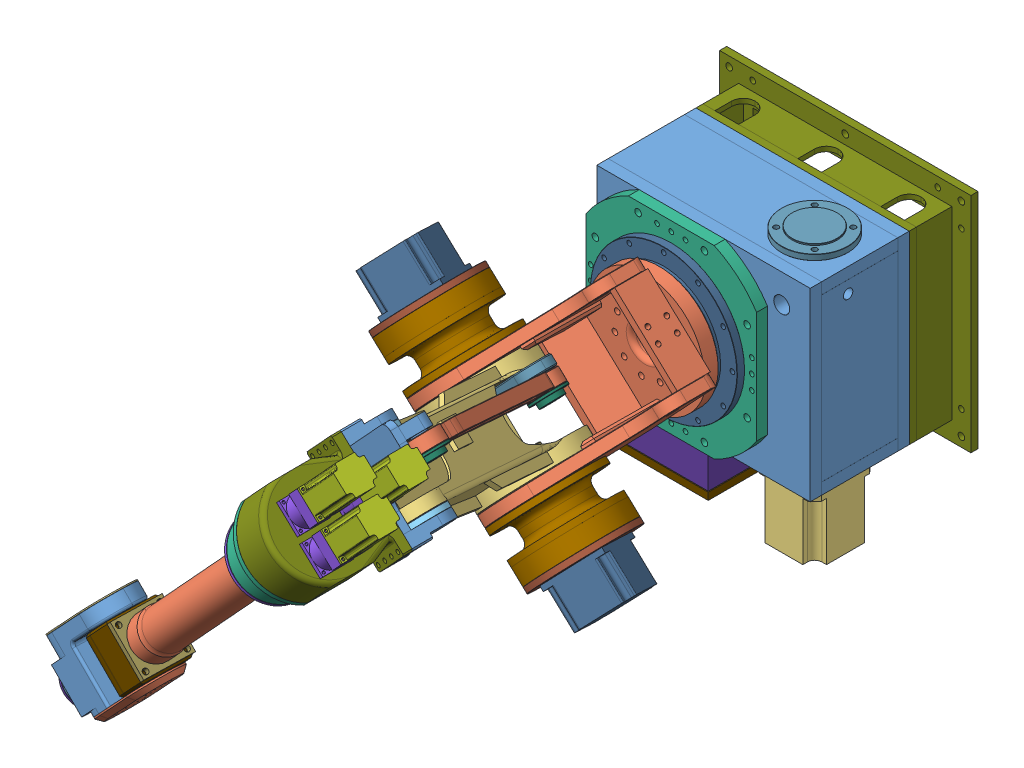
SolidWorks assembly CHX-3装配图, configuration 默认. Lengths in mm. (continued)
Mates (geometry in assembly coordinates): (continued)
- 同心322: concentric aligned: cylinder of CHX-3腕部中心轴2-1 through (-292.5541 -282.9044 1255.4054) axis (0.677165 0.724539 0.128414) radius 7.5; cylinder of CHX-3手腕61902轴承-2 through (-274.4738 -263.5592 1258.8341) axis (0.677165 0.724539 0.128414) radius 14
- 重合247: coincident anti-aligned: plane of CHX-3手腕61902轴承-1 through (-269.7336 -258.4875 1259.733) normal (-0.677165 -0.724539 -0.128414); plane of CHX-3手腕61902轴承-2
- 同心323: concentric anti-aligned: cylinder of CHX-3腕部中心轴1-2 through (-228.9006 -214.7978 1267.4764) axis (-0.677165 -0.724539 -0.128414) radius 34; cylinder of CHK-3前爪固定座-2 through (-246.5068 -233.6358 1264.1376) axis (0.677165 0.724539 0.128414) radius 34
- 同心324: concentric aligned: cylinder of CHK-3前爪固定座-2 through (-241.2095 -229.1944 1226.7182) axis (-0.677165 -0.724539 -0.128414) radius 3; cylinder of CHX-3腕部中心轴1-2 through (-232.4063 -219.7754 1228.3876) axis (-0.677165 -0.724539 -0.128414) radius 2
- 重合248: coincident anti-aligned: plane of CHX-3腕部中心轴1-2 through (-246.5068 -233.6358 1264.1376) normal (-0.677165 -0.724539 -0.128414); plane of CHK-3前爪固定座-2 through (-215.2712 -271.8091 1314.8045) normal (0.677165 0.724539 0.128414)
- 同心328: concentric anti-aligned: cylinder of CHX-3腕部中心轴2-1 through (-292.5541 -282.9044 1255.4054) axis (0.677165 0.724539 0.128414) radius 7.5; cylinder of CHX-3手腕小齿-1 through (-274.4738 -263.5592 1258.8341) axis (-0.677165 -0.724539 -0.128414) radius 16
- 重合254: coincident anti-aligned: plane of CHX-3手腕61902轴承-2; plane of CHX-3手腕小齿-1 through (-274.4738 -263.5592 1258.8341) normal (0.677165 0.724539 0.128414)
- 重合261: coincident anti-aligned: plane of CHK-3前爪固定座-2 through (-223.3972 -280.5036 1313.2635) normal (-0.677165 -0.724539 -0.128414); plane of CHK-3前爪法兰-1 through (-306.234 -203.5239 1315.7509) normal (0.677165 0.724539 0.128414)
- 同心334: concentric aligned: cylinder of CHK-3前爪固定座-2 through (-254.6328 -242.3303 1262.5966) axis (0.677165 0.724539 0.128414) radius 30.5; cylinder of CHK-3前爪法兰-1 through (-293.2313 -283.629 1255.277) axis (0.677165 0.724539 0.128414) radius 42.5
- 重合264: coincident: plane of CHK-3前爪固定座-2 through (-223.3972 -280.5036 1313.2635) normal (-0.103765 -0.078746 0.99148); line of CHK-3前爪法兰-1 through (-296.245 -212.0315 1311.0777) axis (0.728478 -0.68472 0.021858)
- 同心336: concentric aligned: cylinder of CHK-3前爪法兰-1 through (-263.3637 -311.7025 1256.1732) axis (-0.728478 0.68472 -0.021858) radius 42.5; cylinder of CHX-3手腕前端旋转法兰-1 through (-341.3108 -238.4374 1253.8344) axis (-0.728478 0.68472 -0.021858) radius 47.75
- 距离41: distance = 1 mm anti-aligned: plane of CHK-3前爪法兰-1 through (-376.2015 -295.1143 1190.2088) normal (-0.728478 0.68472 -0.021858); plane of CHX-3手腕前端旋转法兰-1 through (-289.071 -201.0754 1186.4442) normal (0.728478 -0.68472 0.021858)
- 同心338: concentric anti-aligned: cylinder of CHX-3手腕前端旋转法兰-1 through (-282.652 -416.9987 1254.0099) axis (-0.728478 0.68472 -0.021858) radius 27.5; cylinder of CHK-3前爪法兰侧盖-1 through (-314.705 -386.871 1253.0482) axis (0.728478 -0.68472 0.021858) radius 55
- 同心340: concentric aligned: cylinder of CHX-3手腕前端旋转法兰-1 through (-282.652 -416.9987 1254.0099) axis (-0.728478 0.68472 -0.021858) radius 27.5; cylinder of CHK-3前爪法兰侧钣金盖-1 through (-417.4204 -290.3254 1249.9662) axis (-0.728478 0.68472 -0.021858) radius 55
- 重合267: coincident anti-aligned: plane of CHX-3手腕前端旋转法兰-1 through (-320.5842 -185.3703 1310.4408) normal (-0.728478 0.68472 -0.021858); plane of CHK-3前爪法兰侧钣金盖-1 through (-417.4204 -290.3254 1249.9662) normal (0.728478 -0.68472 0.021858)
- 同心341: concentric aligned: cylinder of CHX-3手腕前端旋转法兰-1 through (-355.8804 -224.743 1253.3972) axis (-0.728478 0.68472 -0.021858) radius 55; cylinder of CHK-3前爪法兰侧钣金盖-1 through (-355.8804 -224.743 1253.3972) axis (-0.728478 0.68472 -0.021858) radius 55
- 同心342: concentric anti-aligned: cylinder of CHX-3手腕前端旋转法兰-1 through (-323.0988 -255.5554 1254.3808) axis (-0.728478 0.68472 -0.021858) radius 17.5; cylinder of CHX-3小手腕旋转齿轮-2 through (-371.1784 -210.3639 1252.9382) axis (0.728478 -0.68472 0.021858) radius 8.5
- 同心344: concentric aligned: cylinder of CHX-3手腕前端旋转法兰-1 through (-323.0988 -255.5554 1254.3808) axis (-0.728478 0.68472 -0.021858) radius 17.5; cylinder of CHX-3手腕大齿-2-1 through (-324.5558 -254.186 1254.3371) axis (-0.728478 0.68472 -0.021858) radius 27.5
- 重合271: coincident aligned: plane of CHK-3前爪法兰-1 through (-324.5558 -254.186 1254.3371) normal (-0.728478 0.68472 -0.021858); plane of CHX-3手腕大齿-2-1 through (-324.5558 -254.186 1254.3371) normal (-0.728478 0.68472 -0.021858)
- 同心345: concentric aligned: cylinder of CHX-3手腕前端旋转法兰-1 through (-337.9277 -242.8472 1277.4428) axis (-0.728478 0.68472 -0.021858) radius 5; cylinder of CHX-3手腕大齿-2-1 through (-323.3581 -256.5416 1277.88) axis (-0.728478 0.68472 -0.021858) radius 2
- 距离44: distance = 1 mm anti-aligned: plane of CHX-3手腕前端旋转法兰-1 through (-341.3108 -238.4374 1253.8344) normal (-0.728478 0.68472 -0.021858); plane of CHX-3小手腕旋转齿轮-2 through (-342.0393 -237.7527 1253.8125) normal (0.728478 -0.68472 0.021858)
- 同心347: concentric aligned: cylinder of CHX-3手腕大齿-2-1 through (-315.8141 -262.4026 1254.5994) axis (0.728478 -0.68472 0.021858) radius 17; cylinder of CHX-3手腕轴1-1 through (-352.9664 -227.4819 1253.4846) axis (0.728478 -0.68472 0.021858) radius 8.5
- 同心348: concentric aligned: cylinder of CHK-3前爪法兰-1 through (-261.9067 -313.072 1256.2169) axis (0.728478 -0.68472 0.021858) radius 45; cylinder of CHK-3前爪法兰侧盖-1 through (-253.165 -321.2886 1256.4792) axis (0.728478 -0.68472 0.021858) radius 55
- 同心349: concentric anti-aligned: cylinder of CHK-3前爪法兰-1 through (-261.9067 -313.072 1256.2169) axis (0.728478 -0.68472 0.021858) radius 45; cylinder of CHX-3手腕前爪连接轴-1 through (-253.8934 -320.6039 1256.4573) axis (-0.728478 0.68472 -0.021858) radius 27.5
- 重合277: coincident anti-aligned: plane of CHK-3前爪法兰-1 through (-261.9067 -313.072 1256.2169) normal (0.728478 -0.68472 0.021858); plane of CHX-3手腕前爪连接轴-1 through (-261.9067 -313.072 1256.2169) normal (-0.728478 0.68472 -0.021858)
- 重合278: coincident anti-aligned: plane of CHK-3前爪法兰侧盖-1 through (-248.0656 -326.0817 1256.6322) normal (-0.728478 0.68472 -0.021858); plane of CHX-3手腕前爪连接轴-1 through (-248.0656 -326.0817 1256.6322) normal (0.728478 -0.68472 0.021858)
- 同心350: concentric aligned: cylinder of CHK-3前爪法兰侧盖-1 through (-250.8925 -292.5681 1256.9435) axis (0.728478 -0.68472 0.021858) radius 3; cylinder of CHX-3手腕前爪连接轴-1 through (-243.6078 -299.4153 1257.1621) axis (0.728478 -0.68472 0.021858) radius 2.5
- 重合279: coincident aligned: plane of CHX-3手腕大齿-2-1 through (-315.8141 -262.4026 1254.5994) normal (-0.728478 0.68472 -0.021858); plane of CHX-3手腕轴1-1 through (-315.8141 -262.4026 1254.5994) normal (-0.728478 0.68472 -0.021858)
- 齿轮配合14: gear = 0.001 : 0.001: cone of CHX-3手腕大齿2-1 through (-267.0771 -255.6451 1260.2367) axis (-0.677165 -0.724539 -0.128414); cone of CHX-3手腕大齿-2-1 through (-321.2944 -257.2515 1254.435) axis (0.728478 -0.68472 0.021858)
- 重合281: coincident aligned: plane of CHX-3小手腕旋转齿轮-2 through (-363.376 -216.9427 1244.316) normal (0.638355 0.690038 0.341101); plane of CHX-3手腕轴1-1 through (-341.3661 -237.3375 1244.3834) normal (0.638355 0.690038 0.341101)
- 同心352: concentric anti-aligned: cylinder of CHX-3手腕前端旋转法兰-1 through (-358.1902 -352.8548 1251.6553) axis (-0.683779 -0.728693 -0.038123) radius 30; cylinder of CHX-3手腕前端锥齿2-1 through (-380.0711 -376.173 1250.4354) axis (0.683779 0.728693 0.038123) radius 19.9123
- 距离45: distance = 18 mm aligned: plane of CHX-3手腕前端旋转法兰-1 through (-427.4724 -359.1824 1303.7125) normal (-0.683779 -0.728693 -0.038123); plane of CHX-3手腕前端锥齿2-1 through (-380.0711 -376.173 1250.4354) normal (-0.683779 -0.728693 -0.038123)
- 同心354: concentric aligned: cylinder of CHX-3手腕前端旋转法兰-1 through (-282.652 -416.9987 1254.0099) axis (-0.728478 0.68472 -0.021858) radius 27.5; cylinder of CHX-3小手腕旋转齿轮-2-1 through (-385.3674 -320.4531 1250.9279) axis (-0.728478 0.68472 -0.021858) radius 17.5
- 重合284: coincident aligned: plane of CHX-3小手腕旋转齿轮-2 through (-352.9664 -227.4819 1253.4846) normal (-0.728478 0.68472 -0.021858); plane of CHX-3小手腕旋转齿轮-2-1 through (-414.5065 -293.0643 1250.0536) normal (-0.728478 0.68472 -0.021858)
- 齿轮配合16: gear = 0.094 : 0.094: cylinder of CHX-3小手腕旋转齿轮-2 through (-342.0393 -237.7527 1253.8125) axis (-0.728478 0.68472 -0.021858) radius 47; cylinder of CHX-3小手腕旋转齿轮-2-1 through (-414.5065 -293.0643 1250.0536) axis (0.728478 -0.68472 0.021858) radius 47
- 同心357: concentric aligned: cylinder of CHX-3手腕前端旋转法兰-1 through (-282.652 -416.9987 1254.0099) axis (-0.728478 0.68472 -0.021858) radius 27.5; cylinder of CHX-3小手腕锥齿轮旋转中心轴-1 through (-381.725 -323.8767 1251.0372) axis (-0.728478 0.68472 -0.021858) radius 17.5
- 重合286: coincident aligned: plane of CHX-3小手腕旋转齿轮-2-1 through (-414.5065 -293.0643 1250.0536) normal (-0.728478 0.68472 -0.021858); plane of CHX-3小手腕锥齿轮旋转中心轴-1 through (-414.5065 -293.0643 1250.0536) normal (-0.728478 0.68472 -0.021858)
- 同心358: concentric anti-aligned: cylinder of CHX-3手腕前端旋转法兰-1 through (-331.46 -371.1224 1252.5454) axis (0.728478 -0.68472 0.021858) radius 23.5; cylinder of CHX-3手腕6204轴承-1 through (-318.3474 -383.4474 1252.9389) axis (-0.728478 0.68472 -0.021858) radius 23.5
- 重合287: coincident anti-aligned: plane of CHX-3手腕前端旋转法兰-1 through (-328.5461 -373.8613 1252.6329) normal (0.728478 -0.68472 0.021858); plane of CHX-3手腕6204轴承-1 through (-328.5461 -373.8613 1252.6329) normal (-0.728478 0.68472 -0.021858)
- 同心359: concentric anti-aligned: cylinder of CHX-3手腕前端旋转法兰-1 through (-395.5661 -310.867 1250.6219) axis (-0.728478 0.68472 -0.021858) radius 31; cylinder of CHX-3手腕6007轴承-1 through (-402.1224 -304.7045 1250.4252) axis (0.728478 -0.68472 0.021858) radius 17.5
- 重合288: coincident anti-aligned: plane of CHX-3手腕前端旋转法兰-1 through (-395.5661 -310.867 1250.6219) normal (-0.728478 0.68472 -0.021858); plane of CHX-3手腕6007轴承-1 through (-395.5661 -310.867 1250.6219) normal (0.728478 -0.68472 0.021858)
- 同心360: concentric anti-aligned: cylinder of CHK-3前爪法兰-1 through (-261.9067 -313.072 1256.2169) axis (0.728478 -0.68472 0.021858) radius 45; cylinder of CHX-3手腕16011轴承-1 through (-253.8934 -320.6039 1256.4573) axis (-0.728478 0.68472 -0.021858) radius 27.5
- 重合289: coincident anti-aligned: plane of CHK-3前爪法兰-1 through (-261.9067 -313.072 1256.2169) normal (0.728478 -0.68472 0.021858); plane of CHX-3手腕16011轴承-1 through (-261.9067 -313.072 1256.2169) normal (-0.728478 0.68472 -0.021858)
- 同心361: concentric aligned: cylinder of CHK-3前爪法兰-1 through (-324.5558 -254.186 1254.3371) axis (-0.728478 0.68472 -0.021858) radius 45; cylinder of CHX-3手腕16011轴承-2 through (-324.5558 -254.186 1254.3371) axis (-0.728478 0.68472 -0.021858) radius 27.5
- 重合290: coincident anti-aligned: plane of CHK-3前爪法兰-1 through (-324.5558 -254.186 1254.3371) normal (-0.728478 0.68472 -0.021858); plane of CHX-3手腕16011轴承-2 through (-324.5558 -254.186 1254.3371) normal (0.728478 -0.68472 0.021858)
- 同心362: concentric aligned: cylinder of CHX-3手腕前端旋转法兰-1 through (-375.2847 -371.0721 1250.7023) axis (-0.683779 -0.728693 -0.038123) radius 34; cylinder of CHX-3小手腕前端法兰-1 through (-376.6523 -372.5295 1250.626) axis (-0.683779 -0.728693 -0.038123) radius 34
- 重合292: coincident anti-aligned: plane of CHX-3手腕前端旋转法兰-1 through (-427.4724 -359.1824 1303.7125) normal (-0.683779 -0.728693 -0.038123); plane of CHX-3小手腕前端法兰-1 through (-392.3792 -389.2895 1249.7492) normal (0.683779 0.728693 0.038123)
- 同心364: concentric anti-aligned: cylinder of CHX-3手腕前端旋转法兰-1 through (-352.9834 -405.7479 1251.1954) axis (-0.683779 -0.728693 -0.038123) radius 2.5; cylinder of CHX-3小手腕前端法兰-1 through (-380.3345 -434.8956 1249.6705) axis (0.683779 0.728693 0.038123) radius 3
- 同心365: concentric anti-aligned: cylinder of CHX-3手腕前端锥齿2-1 through (-344.3095 -338.0623 1252.4292) axis (-0.683779 -0.728693 -0.038123) radius 10; cylinder of CHX-3腕部前端中心轴-1 through (-380.0711 -376.173 1250.4354) axis (0.683779 0.728693 0.038123) radius 10
- 同心371: concentric aligned: cylinder of CHX-3手腕轴1-1 through (-313.4101 -264.6622 1254.6715) axis (0.728478 -0.68472 0.021858) radius 7; cylinder of CHX-3手腕小齿-2 through (-313.4101 -264.6622 1254.6715) axis (0.728478 -0.68472 0.021858) radius 16
- 重合300: coincident anti-aligned: plane of CHX-3手腕轴1-1 through (-313.4101 -264.6622 1254.6715) normal (0.728478 -0.68472 0.021858); plane of CHX-3手腕小齿-2 through (-313.4101 -264.6622 1254.6715) normal (-0.728478 0.68472 -0.021858)
- 重合301: coincident aligned: plane of CHX-3手腕轴1-1 through (-310.0737 -261.2954 1248.9459) normal (-0.638355 -0.690038 -0.341101); plane of CHX-3手腕小齿-2 through (-309.8123 -261.0488 1247.9577) normal (-0.638355 -0.690038 -0.341101)
- 齿轮配合18: gear = 0.001 : 0.001: cone of CHX-3手腕小齿-1 through (-280.7519 -270.2766 1257.6435) axis (-0.677165 -0.724539 -0.128414); cone of CHX-3手腕小齿-2 through (-306.6563 -271.0104 1254.8742) axis (0.728478 -0.68472 0.021858)
- 重合305: coincident anti-aligned: plane of CHX-3小手臂旋转轴承法兰-1 through (56.8632 90.9578 1321.6672) normal (-0.677165 -0.724539 -0.128414); plane of CHX-3小手臂骨架油封-1 through (56.8632 90.9578 1321.6672) normal (0.677165 0.724539 0.128414)
- 同心374: concentric anti-aligned: cylinder of CHX-3小手臂旋转轴承法兰-1 through (56.8632 90.9578 1321.6672) axis (-0.677165 -0.724539 -0.128414) radius 52.5; cylinder of CHX-3小手臂骨架油封-1 through (48.7372 82.2633 1320.1263) axis (0.677165 0.724539 0.128414) radius 52.5
- 同心379: concentric aligned: cylinder of CHX-3小手腕前端法兰-1 through (-380.0711 -376.173 1250.4354) axis (-0.683779 -0.728693 -0.038123) radius 27.5; cylinder of CHX-3手腕前端轴承顶套-1 through (-397.8494 -395.119 1249.4442) axis (-0.683779 -0.728693 -0.038123) radius 27.5
- 重合307: coincident anti-aligned: plane of CHX-3小手腕前端法兰-1 through (-399.2169 -396.5764 1249.368) normal (-0.683779 -0.728693 -0.038123); plane of CHX-3手腕前端轴承顶套-1 through (-399.2169 -396.5764 1249.368) normal (0.683779 0.728693 0.038123)
- 同心381: concentric aligned: cylinder of CHX-3腕部前端中心轴-1 through (-373.5744 -369.2306 1237.2883) axis (-0.683779 -0.728693 -0.038123) radius 3; cylinder of CHX-3手腕前端锥齿2-1 through (-369.4717 -364.8585 1237.5171) axis (-0.683779 -0.728693 -0.038123) radius 2
- 同心382: concentric aligned: cylinder of CHX-3小手腕锥齿轮旋转中心轴-1 through (-308.8772 -392.3487 1253.223) axis (-0.728478 0.68472 -0.021858) radius 10; cylinder of CHX-3手腕前端锥齿1-1 through (-343.6256 -359.6876 1252.1804) axis (-0.728478 0.68472 -0.021858) radius 10
- 重合308: coincident anti-aligned: plane of CHX-3小手腕锥齿轮旋转中心轴-1 through (-381.725 -323.8767 1251.0372) normal (0.728478 -0.68472 0.021858); plane of CHX-3手腕前端锥齿1-1 through (-381.725 -323.8767 1251.0372) normal (-0.728478 0.68472 -0.021858)
- 重合309: coincident aligned: plane of CHX-3小手腕锥齿轮旋转中心轴-1 through (-370.0123 -336.0042 1258.5195) normal (0.655459 0.687358 -0.312909); plane of CHX-3手腕前端锥齿1-1 through (-352.0619 -350.2992 1264.7194) normal (0.655459 0.687358 -0.312909)
- 齿轮配合19: gear = 0.001 : 0.001: cone of CHX-3手腕前端锥齿1-1 through (-371.8894 -333.1215 1251.3323) axis (0.728478 -0.68472 0.021858); cone of CHX-3手腕前端锥齿2-1 through (-370.839 -366.3344 1250.9501) axis (0.683779 0.728693 0.038123)
- 重合311: coincident aligned: plane of CHX-3腕部前端中心轴-1 through (-397.8494 -395.119 1249.4442) normal (0.683779 0.728693 0.038123); plane of CHX-3手腕前端轴承顶套-1 through (-397.8494 -395.119 1249.4442) normal (0.683779 0.728693 0.038123)
- 同心384: concentric anti-aligned: cylinder of CHX-3小手腕前端法兰-1 through (-438.6127 -380.118 1247.9218) axis (0.683779 0.728693 0.038123) radius 3; cylinder of CHX-3手腕前端轴承顶套-1 through (-427.6723 -368.4589 1248.5318) axis (-0.683779 -0.728693 -0.038123) radius 3
- 重合312: coincident aligned: plane of CHX-3手腕前端轴承顶套-1 through (-408.7899 -406.7781 1248.8343) normal (-0.683779 -0.728693 -0.038123); plane of CHX-3腕部中心轴骨架油封-2 through (-408.7899 -406.7781 1248.8343) normal (-0.683779 -0.728693 -0.038123)
- 同心386: concentric aligned: cylinder of CHX-3手腕前端轴承顶套-1 through (-401.9521 -399.4912 1249.2155) axis (-0.683779 -0.728693 -0.038123) radius 27.5; cylinder of CHX-3腕部中心轴骨架油封-2 through (-395.1143 -392.2042 1249.5967) axis (-0.683779 -0.728693 -0.038123) radius 20
- 重合313: coincident anti-aligned: plane of CHX-3小手腕前端法兰-1 through (-380.0711 -376.173 1250.4354) normal (-0.683779 -0.728693 -0.038123); plane of CHX-3手腕61907轴承-1 through (-380.0711 -376.173 1250.4354) normal (0.683779 0.728693 0.038123)
- 同心387: concentric aligned: cylinder of CHX-3小手腕前端法兰-1 through (-380.0711 -376.173 1250.4354) axis (-0.683779 -0.728693 -0.038123) radius 27.5; cylinder of CHX-3手腕61907轴承-1 through (-380.0711 -376.173 1250.4354) axis (-0.683779 -0.728693 -0.038123) radius 27.5
- 重合314: coincident anti-aligned: plane of CHX-3手腕前端轴承顶套-1 through (-397.8494 -395.119 1249.4442) normal (0.683779 0.728693 0.038123); plane of CHX-3手腕61907轴承-2 through (-397.8494 -395.119 1249.4442) normal (-0.683779 -0.728693 -0.038123)
- 同心388: concentric aligned: cylinder of CHX-3小手腕前端法兰-1 through (-380.0711 -376.173 1250.4354) axis (-0.683779 -0.728693 -0.038123) radius 27.5; cylinder of CHX-3手腕61907轴承-2 through (-391.0116 -387.8321 1249.8255) axis (-0.683779 -0.728693 -0.038123) radius 27.5
- 同心389: concentric aligned: cylinder of CHX-3驱动臂座-1 through (16.2261 47.4792 488.5814) axis (0 0 -1) radius 125; cylinder of CHX-3底盘旋转涡轮轴-1 through (16.2261 47.4792 462.5814) axis (0 0 -1) radius 80
- 同心390: concentric anti-aligned: cylinder of CHX-3底盘旋转涡轮-1 through (16.2261 47.4792 327.5814) axis (0 0 -1) radius 38; cylinder of CHX-3底盘旋转涡轮箱-1 through (16.2261 47.4792 367.5814) axis (0 0 1) radius 157.5
- 同心391: concentric aligned: cylinder of CHX-3底盘旋转电机SGMGH-13A-B键8X7-1 through (191.2261 -112.5208 306.0814) axis (0 -1 0) radius 11; circle of CHX-3底盘旋转涡轮箱-1
- 平行14: parallel aligned: plane of CHX-3底盘旋转涡轮箱-1 through (286.2261 242.4792 225.5814) normal (1 0 0); plane of CHX-3底盘旋转电机SGMGH-13A-B键8X7-1 through (256.2261 -309.5208 371.0814) normal (1 0 0)
- 同心392: concentric aligned: cylinder of CHX-3底盘旋转电机SGMGH-13A-B键8X7-1 through (191.2261 -112.5208 306.0814) axis (0 -1 0) radius 11; cylinder of CHX-3底盘旋转涡杆-1 through (191.2261 133.4792 306.0814) axis (0 -1 0) radius 29
- 齿轮配合20: gear = 0.060005 : 0.312267: cylinder of CHX-3底盘旋转涡轮-1 through (16.2261 47.4792 269.0814) axis (0 0 -1) radius 156.1336; cylinder of CHX-3底盘旋转涡杆-1 through (191.2261 -89.0208 306.0814) axis (0 -1 0) radius 30.0027
- 距离47: distance = 86 mm aligned: plane of CHX-3底盘旋转涡轮箱-1 through (-163.7739 -147.5208 410.5814) normal (0 0 1); plane of CHX-3底盘旋转涡轮-1 through (16.2261 47.4792 324.5814) normal (0 0 1)
- 重合317: coincident aligned: plane of CHX-3底盘旋转涡轮箱-1 through (-163.7739 242.4792 225.5814) normal (-1 0 0); plane of CHX-3底盘法兰盖-1 through (-163.7739 242.4792 433.5814) normal (-1 0 0)
- 重合318: coincident aligned: plane of CHX-3底盘旋转涡轮箱-1 through (-163.7739 -147.5208 225.5814) normal (0 -1 0); plane of CHX-3底盘法兰盖-1 through (-163.7739 -147.5208 433.5814) normal (0 -1 0)
- 重合319: coincident anti-aligned: plane of CHX-3底盘旋转涡轮箱-1 through (-163.7739 -147.5208 410.5814) normal (0 0 1); plane of CHX-3底盘法兰盖-1 through (-163.7739 -147.5208 410.5814) normal (0 0 -1)
- 同心394: concentric anti-aligned: cylinder of CHX-3底盘旋转涡轮-1 through (16.2261 47.4792 356.0814) axis (0 0 -1) radius 60; cylinder of CHX-3底盘旋转涡轮轴-1 through (16.2261 47.4792 257.0814) axis (0 0 1) radius 38
- 重合324: coincident anti-aligned: plane of CHX-3驱动臂座-1 through (16.2261 47.4792 459.5814) normal (0 0 -1); plane of CHX-3底盘旋转涡轮轴-1 through (16.2261 47.4792 459.5814) normal (0 0 1)
- 同心395: concentric anti-aligned: cylinder of CHX-3驱动臂座-1 through (24.22 111.9858 499.5814) axis (0 0 -1) radius 6; cylinder of CHX-3底盘旋转涡轮轴-1 through (24.22 111.9858 432.5814) axis (0 0 1) radius 5
- 同心398: concentric aligned: cylinder of CHX-3底盘旋转涡轮轴-1 through (16.2261 47.4792 130.5814) axis (0 0 1) radius 37.5; cylinder of CHX-3底盘旋转涡轮轴下法兰-1 through (16.2261 47.4792 177.0814) axis (0 0 1) radius 47.5
- 重合327: coincident aligned: plane of CHX-3底盘旋转涡轮-1 through (-22.0174 69.5345 326.9875) normal (0.682819 0.730588 0); plane of CHX-3底盘旋转涡轮轴-1 through (-13.2503 61.3407 271.0814) normal (0.682819 0.730588 0)
- 同心399: concentric anti-aligned: cylinder of CHX-3底盘旋转涡轮箱-1 through (-71.7466 18.8951 219.5814) axis (0 0 -1) radius 4; cylinder of CHX-3底盘旋转涡轮轴下法兰-1 through (-71.7466 18.8951 169.5814) axis (0 0 1) radius 5
- 同心403: concentric aligned: cylinder of CHX-3底盘旋转涡轮轴下法兰-1 through (16.2261 47.4792 212.0814) axis (0 0 1) radius 67.5; cylinder of CHX-3底盘旋转51315轴承-2 through (16.2261 47.4792 212.0814) axis (0 0 1) radius 67.5
- 重合330: coincident anti-aligned: plane of CHX-3底盘旋转涡轮轴下法兰-1 through (16.2261 47.4792 212.0814) normal (0 0 1); plane of CHX-3底盘旋转51315轴承-2 through (16.2261 47.4792 212.0814) normal (0 0 -1)
- 同心404: concentric aligned: cylinder of CHX-3底盘法兰盖-1 through (16.2261 47.4792 403.5814) axis (0 0 1) radius 135; cylinder of CHX-3底盘旋转涡轮轴上法兰盖-1 through (16.2261 47.4792 389.5814) axis (0 0 1) radius 135
- 重合331: coincident anti-aligned: plane of CHX-3底盘法兰盖-1 through (-163.7739 -147.5208 433.5814) normal (0 0 1); circle of CHX-3底盘旋转涡轮轴上法兰盖-1
- 同心405: concentric anti-aligned: cylinder of CHX-3底盘旋转涡轮轴上法兰盖-1 through (16.2261 47.4792 389.5814) axis (0 0 1) radius 120; cylinder of CHX-3底盘旋转涡轮轴上法兰16032轴承-2 through (16.2261 47.4792 434.5814) axis (0 0 -1) radius 80
- 重合332: coincident anti-aligned: plane of CHX-3底盘旋转涡轮轴上法兰盖-1 through (16.2261 47.4792 434.5814) normal (0 0 -1); plane of CHX-3底盘旋转涡轮轴上法兰16032轴承-2 through (16.2261 47.4792 434.5814) normal (0 0 1)
- 重合334: coincident anti-aligned: plane of CHX-3底盘旋转涡轮箱-1 through (-163.7739 -147.5208 201.5814) normal (0 0 -1); plane of CHX-3底盘旋转涡轮轴下法兰-1 through (16.2261 47.4792 201.5814) normal (0 0 1)
- 同心410: concentric aligned: cylinder of CHX-3底盘旋转涡轮轴下法兰-1 through (16.2261 47.4792 193.5814) axis (0 0 -1) radius 57.5; cylinder of CHX-3底盘旋转涡轮轴下法兰6215轴承-2 through (16.2261 47.4792 193.5814) axis (0 0 -1) radius 37.5
- 重合337: coincident anti-aligned: plane of CHX-3底盘旋转涡轮轴下法兰-1 through (16.2261 47.4792 193.5814) normal (0 0 -1); plane of CHX-3底盘旋转涡轮轴下法兰6215轴承-2 through (16.2261 47.4792 193.5814) normal (0 0 1)
- 重合338: coincident anti-aligned: plane of CHX-3底盘旋转涡轮轴下法兰6215轴承-1 through (16.2261 47.4792 173.5814) normal (0 0 1); plane of CHX-3底盘旋转涡轮轴下法兰6215轴承-2 through (16.2261 47.4792 173.5814) normal (0 0 -1)
- 同心411: concentric aligned: cylinder of CHX-3底盘旋转涡轮轴下法兰-1 through (16.2261 47.4792 193.5814) axis (0 0 -1) radius 57.5; cylinder of CHX-3底盘旋转涡轮轴下法兰6215轴承-1 through (16.2261 47.4792 173.5814) axis (0 0 -1) radius 57.5
- 重合340: coincident anti-aligned: plane of CHX-3底盘旋转涡轮-1 through (16.2261 47.4792 356.0814) normal (0 0 1); plane of CHX-3底盘旋转涡轮轴-1 through (16.2261 47.4792 356.0814) normal (0 0 -1)
- 同心412: concentric aligned: cylinder of CHX-3底盘旋转涡轮轴上法兰盖-1 through (16.2261 47.4792 455.5814) axis (0 0 -1) radius 95; cylinder of CHX-3底盘旋转涡轮轴上法兰油封-1 through (16.2261 47.4792 455.5814) axis (0 0 -1) radius 95
- 重合342: coincident aligned: plane of CHX-3底盘旋转涡轮轴上法兰盖-1 through (16.2261 47.4792 455.5814) normal (0 0 1); plane of CHX-3底盘旋转涡轮轴上法兰油封-1 through (16.2261 47.4792 455.5814) normal (0 0 1)
- 距离48: distance = 34 mm aligned: plane of CHX-3底盘旋转涡轮箱-1 through (-163.7739 242.4792 386.5814) normal (0 1 0); plane of CHX-3底盘旋转涡杆-1 through (191.2261 208.4792 306.0814) normal (0 1 0)
- 同心414: concentric aligned: cylinder of CHX-3底盘旋转涡轮箱-1 through (191.2261 -104.5208 306.0814) axis (0 -1 0) radius 47.5; cylinder of CHX-3底盘旋转涡杆电机法兰-1 through (191.2261 -118.5208 306.0814) axis (0 -1 0) radius 47.25
- 同心415: concentric aligned: cylinder of CHX-3底盘旋转涡轮箱-1 through (191.2261 202.2792 306.0814) axis (0 1 0) radius 47.5; cylinder of CHX-3底盘旋转涡杆轴承法兰-1 through (191.2261 213.4792 306.0814) axis (0 1 0) radius 47.25
- 重合346: coincident anti-aligned: plane of CHX-3底盘旋转涡轮箱-1 through (-163.7739 242.4792 386.5814) normal (0 1 0); plane of CHX-3底盘旋转涡杆轴承法兰-1 through (191.2261 242.4792 306.0814) normal (0 -1 0)
- 重合347: coincident anti-aligned: plane of CHX-3底盘旋转涡轮箱-1 through (-163.7739 -147.5208 410.5814) normal (0 -1 0); plane of CHX-3底盘旋转涡杆电机法兰-1 through (191.2261 -147.5208 306.0814) normal (0 1 0)
- 重合348: coincident anti-aligned: plane of CHX-3底盘旋转电机SGMGH-13A-B键8X7-1 through (126.2261 -170.5208 371.0814) normal (0 1 0); plane of CHX-3底盘旋转涡杆电机法兰-1 through (191.2261 -170.5208 306.0814) normal (0 -1 0)
- 同心416: concentric anti-aligned: cylinder of CHX-3底盘旋转涡轮箱-1 through (150.5675 -129.5208 346.74) axis (0 -1 0) radius 5; cylinder of CHX-3底盘旋转涡杆轴承法兰-1 through (150.5675 211.4792 346.74) axis (0 1 0) radius 5.5
- 重合349: coincident anti-aligned: plane of CHX-3轴承1-1 through (129.3199 168.4834 1335.4076) normal (0.677165 0.724539 0.128414); plane of CHX-3小手臂旋转法兰-3 through (129.3199 168.4834 1335.4076) normal (-0.677165 -0.724539 -0.128414)
- 重合350: coincident aligned: plane of CHX-3底盘旋转涡轮箱-1 through (286.2261 242.4792 386.5814) normal (1 0 0); plane of CHX-3箱体底座-1 through (286.2261 -147.5208 111.5814) normal (1 0 0)
- 重合351: coincident aligned: plane of CHX-3底盘旋转涡轮箱-1 through (-163.7739 -147.5208 386.5814) normal (0 -1 0); plane of CHX-3箱体底座-1 through (286.2261 -147.5208 111.5814) normal (0 -1 0)
- 重合352: coincident anti-aligned: plane of CHX-3底盘旋转涡轮箱-1 through (-163.7739 -147.5208 201.5814) normal (0 0 -1); plane of CHX-3箱体底座-1 through (-163.7739 242.4792 201.5814) normal (0 0 1)
- 重合353: coincident anti-aligned: plane of CHX-3底盘旋转涡轮箱-1 through (-163.7739 -147.5208 386.5814) normal (0 -1 0); plane of CHX-3小电箱-1 through (-128.7739 -147.5208 201.5814) normal (0 1 0)
- 重合355: coincident aligned: plane of CHX-3底盘旋转涡轮箱-1 through (-163.7739 -147.5208 410.5814) normal (0 0 1); plane of CHX-3小电箱-1 through (-128.7739 -247.5208 410.5814) normal (0 0 1)
- 重合356: coincident anti-aligned: plane of CHX-3小电箱-1 through (-128.7739 -247.5208 201.5814) normal (0 -1 0); plane of CHX-3小电箱盖-1 through (74.2261 -247.5208 198.5814) normal (0 1 0)
- 距离49: distance = 1 mm anti-aligned: plane of CHX-3小电箱-1 through (-128.7739 -247.5208 410.5814) normal (-1 0 0); plane of CHX-3小电箱盖-1 through (-129.7739 -234.5208 413.5814) normal (1 0 0)
- 距离50: distance = 1 mm anti-aligned: plane of CHX-3小电箱-1 through (-128.7739 -247.5208 201.5814) normal (0 0 -1); plane of CHX-3小电箱盖-1 through (74.2261 -234.5208 200.5814) normal (0 0 1)
- 同心417: concentric anti-aligned: cylinder of CHX-3底盘法兰盖-1 through (16.2261 -97.5208 398.5814) axis (0 0 1) radius 4; cylinder of CHX-3底盘旋转涡轮轴上法兰盖-1 through (16.2261 -97.5208 454.5814) axis (0 0 -1) radius 5
- 同心418: concentric anti-aligned: cylinder of CHX-3底盘旋转涡轮箱-1 through (-93.7739 -127.5208 396.0814) axis (0 -1 0) radius 4; cylinder of CHX-3小电箱-1 through (-93.7739 -169.5208 396.0814) axis (0 1 0) radius 5
- 同心422: concentric anti-aligned: cylinder of CHX-3大手臂2-1 through (-94.7533 -140.0965 609.7219) axis (0.730588 -0.682819 0) radius 4.5; cylinder of CHX-3大手臂摆线减速机手臂安装法兰-1 through (-50.918 -181.0657 609.7219) axis (-0.730588 0.682819 0) radius 4
- 平行15: parallel aligned: plane of CHX-3腕部行星减速机-4 through (297.408 243.5165 1411.8182) normal (0.730588 -0.682819 0); plane of CHX-3腕部电机齿轮箱-1 through (267.7221 184.7616 1284.6703) normal (0.730588 -0.682819 0)
- 平行16: parallel aligned: plane of CHX-3腕部行星减速机-3 through (279.9275 285.6919 1266.0353) normal (0.730588 -0.682819 0); plane of CHX-3腕部电机齿轮箱-1 through (267.7221 184.7616 1284.6703) normal (0.730588 -0.682819 0)
- 平行17: parallel aligned: plane of CHX-3腕部行星减速机-5; plane of CHX-3腕部电机齿轮箱-1 through (267.7221 184.7616 1284.6703) normal (0.730588 -0.682819 0)
- 重合358: coincident anti-aligned: plane of CHX-3腕部电机齿轮箱-1 through (217.9335 109.5221 1231.9436) normal (0.087684 0.093818 -0.991721); plane of CHX-3小手臂座-2 through (84.9665 233.795 1231.9436) normal (-0.087684 -0.093818 0.991721)
- 同心423: concentric aligned: cylinder of CHX-3腕部电机齿轮箱-1 through (269.0635 178.8743 1232.9416) axis (-0.087684 -0.093818 0.991721) radius 4.5; cylinder of CHX-3小手臂座-2 through (269.5019 179.3433 1227.983) axis (-0.087684 -0.093818 0.991721) radius 4
- 同心424: concentric aligned: cylinder of CHX-3腕部电机齿轮箱-1 through (218.2761 124.5338 1223.3106) axis (-0.087684 -0.093818 0.991721) radius 4.5; cylinder of CHX-3小手臂座-2 through (218.7145 125.0029 1218.352) axis (-0.087684 -0.093818 0.991721) radius 4
- 重合360: coincident anti-aligned: plane of CHX-3小手臂关节轴芯-1 through (235.3418 169.1548 1173.5815) normal (0.730588 -0.682819 0); plane of CHX-3小手臂座-2 through (197.4771 128.641 1231.9436) normal (-0.730588 0.682819 0)
- 同心426: concentric aligned: cylinder of CHX-3小手臂关节轴芯-1 through (235.3418 169.1548 1173.5815) axis (-0.730588 0.682819 0) radius 47.5; cylinder of CHX-3小手臂座-2 through (255.7983 150.0358 1173.5815) axis (-0.730588 0.682819 0) radius 47.5
- 同心436: concentric anti-aligned: cylinder of CHX-3小手臂座-2 through (277.2936 341.4559 1206.6991) axis (-0.730588 0.682819 0) radius 12.5; cylinder of CHX-3连杆-2 through (261.2207 356.478 1206.6991) axis (0.730588 -0.682819 0) radius 23.5
- 重合364: coincident aligned: plane of CHX-3小手臂座-2 through (261.2207 356.478 1206.6991) normal (0.730588 -0.682819 0); plane of CHX-3连杆-2 through (261.2207 356.478 1206.6991) normal (0.730588 -0.682819 0)
- 同心437: concentric anti-aligned: cylinder of CHX-3连杆轴传动轴-1 through (5.9513 33.5565 676.9678) axis (-0.730588 0.682819 0) radius 12.5; cylinder of CHX-3连杆-2 through (-18.8887 56.7724 676.9678) axis (0.730588 -0.682819 0) radius 23.5
- 同心438: concentric aligned: cylinder of CHX-3连杆轴承盖-1 through (289.7136 329.848 1206.6991) axis (-0.730588 0.682819 0) radius 23.5; cylinder of CHX-3小手臂座-2 through (277.2936 341.4559 1206.6991) axis (-0.730588 0.682819 0) radius 12.5
- 重合365: coincident anti-aligned: plane of CHX-3连杆轴承盖-1 through (278.7548 340.0903 1206.6991) normal (-0.730588 0.682819 0); plane of CHX-3连杆-2 through (278.7548 340.0903 1206.6991) normal (0.730588 -0.682819 0)
- 同心439: concentric aligned: cylinder of CHX-3连杆轴承盖-1 through (289.8366 362.1991 1188.3308) axis (0.730588 -0.682819 0) radius 3; cylinder of CHX-3连杆-2 through (280.339 371.0757 1188.3308) axis (0.730588 -0.682819 0) radius 2.5
- 同心440: concentric anti-aligned: cylinder of CHX-3连杆轴承盖-2 through (9.6042 30.1424 676.9678) axis (-0.730588 0.682819 0) radius 23.5; cylinder of CHX-3连杆-2 through (-18.8887 56.7724 676.9678) axis (0.730588 -0.682819 0) radius 23.5
- 重合366: coincident anti-aligned: plane of CHX-3连杆轴承盖-2; plane of CHX-3连杆-2 through (278.7548 340.0903 1206.6991) normal (0.730588 -0.682819 0)
- 同心441: concentric aligned: circle of CHX-3连杆轴承盖-2; cylinder of CHX-3连杆-2 through (2.9935 74.3274 688.3251) axis (0.730588 -0.682819 0) radius 2.5
- 同心442: concentric aligned: cylinder of CHX-3小手臂座-2 through (243.2478 195.1881 1205.2637) axis (0.730588 -0.682819 0) radius 3.5; cylinder of CHX-3小手臂关节轴芯-1 through (229.3667 208.1616 1205.2637) axis (0.730588 -0.682819 0) radius 3
- 同心443: concentric aligned: cylinder of CHX-3小手臂旋转法兰-3 through (73.7489 109.0248 1395.4538) axis (-0.677165 -0.724539 -0.128414) radius 2.5; cylinder of CHX-3小手臂旋转轴承法兰-1 through (79.8434 115.5457 1396.6095) axis (-0.677165 -0.724539 -0.128414) radius 3
- 重合367: coincident aligned: plane of CHX-3手腕直齿1-1 through (204.5698 219.1047 1361.6218) normal (0.440791 -0.259684 -0.859225); plane of CHX-3腕部中心轴3-1 through (170.4742 188.9681 1353.2387) normal (0.440791 -0.259684 -0.859225)
- 同心444: concentric aligned: cylinder of CHX-3腕部中心轴3-1 through (-274.4738 -263.5592 1258.8341) axis (0.677165 0.724539 0.128414) radius 20; cylinder of CHX-3手腕大齿2-1 through (-276.2344 -265.4431 1258.5002) axis (0.677165 0.724539 0.128414) radius 20
- 重合370: coincident anti-aligned: plane of CHX-3手腕直齿2-1 through (141.5088 181.5252 1337.719) normal (-0.677165 -0.724539 -0.128414); plane of CHX-3小手臂旋转后法兰-1 through (141.5088 181.5252 1337.719) normal (0.677165 0.724539 0.128414)
- 同心446: concentric anti-aligned: cylinder of CHX-3手腕直齿2-1 through (123.564 162.3249 1334.316) axis (0.677165 0.724539 0.128414) radius 30; cylinder of CHX-3小手臂旋转后法兰-1 through (155.0521 196.0159 1340.2873) axis (-0.677165 -0.724539 -0.128414) radius 30
- 同心448: concentric aligned: cylinder of CHX-3手腕直齿2-1 through (100.2834 193.0537 1334.3201) axis (0.677165 0.724539 0.128414) radius 3; cylinder of CHX-3小手臂旋转后法兰-1 through (107.055 200.2991 1335.6043) axis (0.677165 0.724539 0.128414) radius 3
- 同心449: concentric aligned: cylinder of CHX-3腕部中心轴1-2 through (96.8975 189.4311 1333.6781) axis (0.677165 0.724539 0.128414) radius 2; cylinder of CHX-3手腕直齿2-1 through (123.307 217.6881 1338.6862) axis (0.677165 0.724539 0.128414) radius 4.75
- 重合371: coincident anti-aligned: plane of CHX-3腕部中心轴3-1 through (-257.2738 -245.156 1262.0958) normal (-0.677165 -0.724539 -0.128414); plane of CHX-3手腕大齿2-1 through (-257.2738 -245.156 1262.0958) normal (0.677165 0.724539 0.128414)
- 重合372: coincident aligned: plane of CHX-3腕部中心轴3-1 through (-280.1882 -250.2968 1248.4027) normal (-0.440791 0.259684 0.859225); plane of CHX-3手腕大齿2-1 through (-286.5626 -253.5977 1246.1302) normal (-0.440791 0.259684 0.859225)
- 同心450: concentric anti-aligned: cylinder of CHX-3腕部电机齿轮箱-1 through (233.7642 183.1108 1395.1816) axis (0.677165 0.724539 0.128414) radius 2.5; cylinder of CHX-3腕部行星减速机-4 through (260.8508 212.0924 1400.3181) axis (-0.677165 -0.724539 -0.128414) radius 2.75
- 同心451: concentric anti-aligned: cylinder of CHX-3手腕直齿1-1 through (190.9419 234.4165 1347.0933) axis (-0.677165 -0.724539 -0.128414) radius 22.5; cylinder of CHX-3腕部中心轴3-1 through (-276.1667 -265.3706 1258.513) axis (0.677165 0.724539 0.128414) radius 22.5
- 同心452: concentric aligned: cylinder of CHX-3小手臂旋转法兰-3 through (52.8002 86.6105 1320.8967) axis (0.677165 0.724539 0.128414) radius 62.5; cylinder of CHX-3小手臂旋转法兰轴承隔套-1 through (83.2726 119.2148 1326.6754) axis (0.677165 0.724539 0.128414) radius 50
- 重合373: coincident anti-aligned: plane of CHX-3轴承1-2; plane of CHX-3小手臂旋转法兰轴承隔套-1 through (83.2726 119.2148 1326.6754) normal (-0.677165 -0.724539 -0.128414)
- 重合374: coincident aligned: plane of CHX-3小手腕旋转齿轮-2-1 through (-431.1565 -273.6079 1270.699) normal (0.655459 0.687358 -0.312909); plane of CHX-3小手腕锥齿轮旋转中心轴-1 through (-414.4387 -292.543 1264.1239) normal (0.655459 0.687358 -0.312909)
- 重合375: coincident anti-aligned: plane of CHX-3腕部中心轴2-1 through (158.438 199.6386 1340.9294) normal (0.677165 0.724539 0.128414); plane of CHX-3手腕6002轴承-1 through (158.438 199.6386 1340.9294) normal (-0.677165 -0.724539 -0.128414)
- 同心453: concentric aligned: cylinder of CHX-3腕部中心轴3-1 through (-243.7305 -230.6652 1264.6641) axis (-0.677165 -0.724539 -0.128414) radius 22.45; cylinder of CHX-3腕部中心轴前端锁帽-1 through (-245.1525 -232.1867 1264.3944) axis (-0.677165 -0.724539 -0.128414) radius 21.75
- 重合376: coincident anti-aligned: plane of CHX-3手腕61908轴承-2; plane of CHX-3腕部中心轴前端锁帽-1 through (-245.1525 -232.1867 1264.3944) normal (0.677165 0.724539 0.128414)
- 齿轮配合21: gear = 0.068 : 0.036: cylinder of CHX-3手腕直齿4-1 through (185.3492 167.5537 1364.4739) axis (0.677165 0.724539 0.128414) radius 18; cylinder of CHX-3手腕直齿1-1 through (157.0836 198.1896 1340.6726) axis (0.677165 0.724539 0.128414) radius 34
- 齿轮配合22: gear = 0.098 : 0.036: cylinder of CHX-3手腕直齿4-2 through (147.0329 187.4357 1275.2406) axis (0.677165 0.724539 0.128414) radius 18; cylinder of CHX-3手腕直齿2-1 through (155.0521 196.0159 1340.2873) axis (-0.677165 -0.724539 -0.128414) radius 49
- 齿轮配合23: gear = 0.036 : 0.044: cylinder of CHX-3手腕直齿3-1 through (172.6584 214.854 1343.6261) axis (0.677165 0.724539 0.128414) radius 22; cylinder of CHX-3手腕直齿4-3 through (149.3032 233.0527 1364.1039) axis (0.677165 0.724539 0.128414) radius 18
- 同心454: concentric aligned: cylinder of CHX-3腕部中心轴3-1 through (-243.7305 -230.6652 1264.6641) axis (-0.677165 -0.724539 -0.128414) radius 22.45; cylinder of CHX-3腕部中心轴前端锁帽-2 through (-250.5698 -237.983 1263.3671) axis (-0.677165 -0.724539 -0.128414) radius 21.75
- 重合377: coincident anti-aligned: plane of CHX-3腕部中心轴前端锁帽-1 through (-250.5698 -237.983 1263.3671) normal (-0.677165 -0.724539 -0.128414); plane of CHX-3腕部中心轴前端锁帽-2
- 平行18: parallel aligned: plane of CHK-3前爪法兰-1 through (-305.7152 -203.1301 1310.7936) normal (-0.042031 -0.012825 0.999034); plane of CHX-3手腕前端旋转法兰-1 through (-457.34 -331.1089 1302.8163) normal (-0.042031 -0.012825 0.999034)
